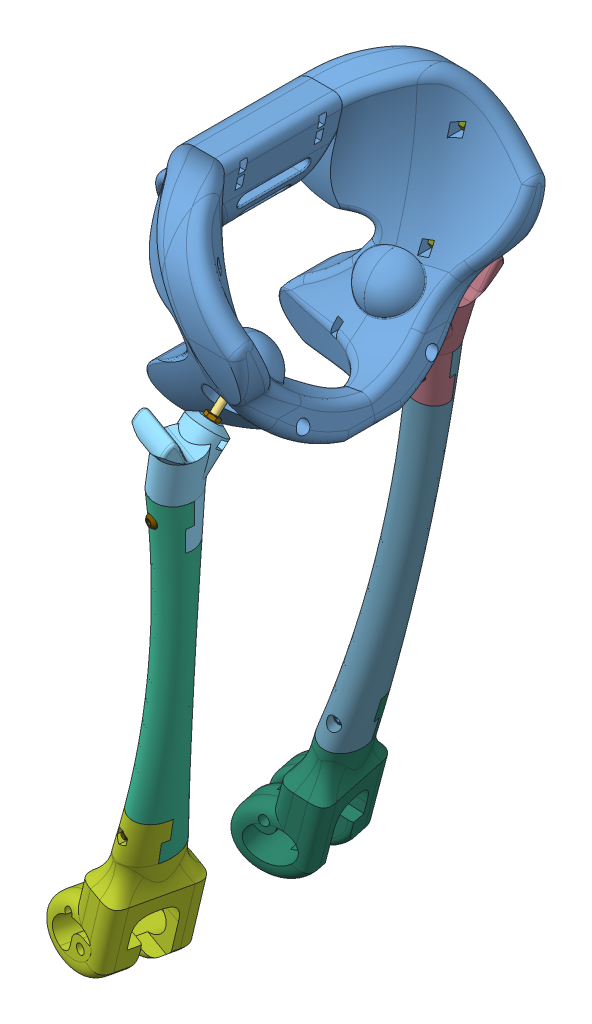
SolidWorks assembly Hips_VerticalCutVer10_Assembly, configuration Default. Lengths in mm.
Overall size (217.51 637.91 297.67).
53 component instances, 21 part files, 66 mates.
Components (placement in the parent):
- IliumRebuilt_Ver10-1: IliumRebuilt_Ver10 [Default] at origin size (197.88 220.17 282.18)
- Femoral_Head_ver1-1: Femoral_Head_ver1 [Default] at (17.9842 -18.1038 8.0845) x (0.971595 0.045629 0.232211) z (-0.227271 -0.093624 0.969321) size (39.5 39.5 39.5)
- 95327A531_HIGH-STRG ZINC YELLOW-CHROMATE PLTD CAP SCREW-1: 95327A531_HIGH-STRG ZINC YELLOW-CHROMATE PLTD CAP SCREW [95327A531] at (-63.8384 -68.3613 80.3964) x (-0.114057 -0.769464 0.628424) z (0.409289 0.539984 0.735459) size (49.38 11.55 10)
- Femoral_Head_Ver1_Cap-1: Femoral_Head_Ver1_Cap [Default] at (17.9868 -18.1069 8.0812) x (0.971595 0.045629 0.232211) z (-0.227271 -0.093624 0.969321) size (19.53 20.18 20.18)
- 03_02_Femoral_Head_Right-1: 03_02_Femoral_Head_Right [Default] at (-72.0104 -117.246 110.2958) x (-0.952156 0.241885 -0.186789) z (0.205625 0.054888 -0.97709) size (46.92 105.86 63.35)
- 03_03_Femur_Right-1: 03_03_Femur_Right [Default] at (-120.2542 -417.7721 83.261) x (-0.952156 0.241885 -0.186789) z (0.205625 0.054888 -0.97709) size (54.81 304.92 50.87)
- 05_01_Knee_Top-1: 05_01_Knee_Top [Default] at (-149.6638 -490.6352 77.3331) x (-0.952156 0.241885 -0.186789) z (0.185137 -0.029753 -0.982262) size (74.55 156.7 74.23)
- 94645A205_HIGH-STRENGTH STEEL NYLON-INSERT LOCKNUT-1: 94645A205_HIGH-STRENGTH STEEL NYLON-INSERT LOCKNUT [94645A205] at (-65.6633 -80.6727 90.4512) x (0.993354 -0.098188 0.060066) z (-0.015485 -0.631098 -0.775548) size (10 6.41 11.55)
- 90695A038_CLASS 04 STEEL THIN HEX NUT - DIN 439B-1: 90695A038_CLASS 04 STEEL THIN HEX NUT - DIN 439B [90695A038] at (-64.7965 -74.8248 85.6752) x (0.993328 -0.099162 0.058868) z (0.017019 0.630946 0.77564) size (10 3.98 11.55)
- MirrorFemoral_Head_ver1-2: MirrorFemoral_Head_ver1 [Default] at (17.9842 -18.1038 -8.0845) x (0.971595 0.045629 -0.232211) z (0.227271 0.093624 0.969321) size (39.5 39.5 39.5)
- Mirror95327A531_HIGH-STRG ZINC YELLOW-CHROMATE PLTD CAP SCREW-2: Mirror95327A531_HIGH-STRG ZINC YELLOW-CHROMATE PLTD CAP SCREW [95327A531] at (-63.8384 -68.3613 -80.3964) x (-0.114057 -0.769464 -0.628424) z (-0.409289 -0.539984 0.735459) size (49.38 11.55 10)
- MirrorFemoral_Head_Ver1_Cap-2: MirrorFemoral_Head_Ver1_Cap [Default] at (17.9868 -18.1069 -8.0812) x (0.971595 0.045629 -0.232211) z (0.227271 0.093624 0.969321) size (19.53 20.18 20.18)
- Mirror03_02_Femoral_Head_Right-2: Mirror03_02_Femoral_Head_Right [Default] at (-72.0104 -117.246 -110.2958) x (-0.952156 0.241885 0.186789) z (-0.205625 -0.054888 -0.97709) size (46.92 105.86 63.35)
- Mirror03_03_Femur_Right-2: Mirror03_03_Femur_Right [Default] at (-120.2542 -417.7721 -83.261) x (-0.952156 0.241885 0.186789) z (-0.205625 -0.054888 -0.97709) size (54.81 304.92 50.87)
- Mirror05_01_Knee_Top-2: Mirror05_01_Knee_Top [Default] at (-149.6638 -490.6352 -77.3331) x (-0.952156 0.241885 0.186789) z (-0.185137 0.029753 -0.982262) size (74.55 156.7 74.23)
- Mirror94645A205_HIGH-STRENGTH STEEL NYLON-INSERT LOCKNUT-2: Mirror94645A205_HIGH-STRENGTH STEEL NYLON-INSERT LOCKNUT [94645A205] at (-65.6633 -80.6727 -90.4512) x (0.993354 -0.098188 -0.060066) z (0.015485 0.631098 -0.775548) size (10 6.41 11.55)
- Mirror90695A038_CLASS 04 STEEL THIN HEX NUT - DIN 439B-2: Mirror90695A038_CLASS 04 STEEL THIN HEX NUT - DIN 439B [90695A038] at (-64.7965 -74.8248 -85.6752) x (0.993328 -0.099162 -0.058868) z (-0.017019 -0.630946 0.77564) size (10 3.98 11.55)
- 91239A330_CLASS 10.9 STL BUTTON-HEAD SOCKET CAP SCREW-1: 91239A330_CLASS 10.9 STL BUTTON-HEAD SOCKET CAP SCREW [91239A330] at (-44.244 -75.4386 54.7323) x (0 0 -1) z (1 0 0) size (10.5 10.5 38.95)
- 91239A330_CLASS 10.9 STL BUTTON-HEAD SOCKET CAP SCREW-4: 91239A330_CLASS 10.9 STL BUTTON-HEAD SOCKET CAP SCREW [91239A330] at (-77.844 52.8275 110.8479) x (0 -0.939693 0.34202) z (-1 0 0) size (10.5 10.5 38.95)
- 91239A330_CLASS 10.9 STL BUTTON-HEAD SOCKET CAP SCREW-6: 91239A330_CLASS 10.9 STL BUTTON-HEAD SOCKET CAP SCREW [91239A330] at (-77.844 -21.0136 84.8541) x (0 -0.866025 0.5) z (-1 0 0) size (10.5 10.5 38.95)
- 91239A330_CLASS 10.9 STL BUTTON-HEAD SOCKET CAP SCREW-8: 91239A330_CLASS 10.9 STL BUTTON-HEAD SOCKET CAP SCREW [91239A330] at (-121.884 56.6312 66.8) x (0.173648 0.984808 0) z (0 0 1) size (10.5 10.5 38.95)
- 91239A330_CLASS 10.9 STL BUTTON-HEAD SOCKET CAP SCREW-10: 91239A330_CLASS 10.9 STL BUTTON-HEAD SOCKET CAP SCREW [91239A330] at (-104.3146 69.6752 66.8) x (-0.173648 0.984808 0) z (0 0 1) size (10.5 10.5 38.95)
- 91239A330_CLASS 10.9 STL BUTTON-HEAD SOCKET CAP SCREW-13: 91239A330_CLASS 10.9 STL BUTTON-HEAD SOCKET CAP SCREW [91239A330] at (-76.9699 -137.6299 128.1216) x (-0.583019 0.808777 -0.077261) z (-0.205625 -0.054888 0.97709) size (10.5 10.5 38.95)
- 91239A330_CLASS 10.9 STL BUTTON-HEAD SOCKET CAP SCREW-15: 91239A330_CLASS 10.9 STL BUTTON-HEAD SOCKET CAP SCREW [91239A330] at (-112.4792 -398.3917 68.7251) x (-0.97858 0.021691 -0.20472) z (0.205625 0.054888 -0.97709) size (10.5 10.5 38.95)
- Mirror91239A330_CLASS 10.9 STL BUTTON-HEAD SOCKET CAP SCREW-17: Mirror91239A330_CLASS 10.9 STL BUTTON-HEAD SOCKET CAP SCREW [91239A330] at (-44.244 -75.4386 -54.7323) x (0 0 1) z (-1 0 0) size (10.5 10.5 38.95)
- Mirror91239A330_CLASS 10.9 STL BUTTON-HEAD SOCKET CAP SCREW-18: Mirror91239A330_CLASS 10.9 STL BUTTON-HEAD SOCKET CAP SCREW [91239A330] at (-77.844 52.8275 -110.8479) x (0 -0.939693 -0.34202) z (1 0 0) size (10.5 10.5 38.95)
- Mirror91239A330_CLASS 10.9 STL BUTTON-HEAD SOCKET CAP SCREW-19: Mirror91239A330_CLASS 10.9 STL BUTTON-HEAD SOCKET CAP SCREW [91239A330] at (-121.884 56.6312 -66.8) x (0.173648 0.984808 0) z (0 0 1) size (10.5 10.5 38.95)
- Mirror91239A330_CLASS 10.9 STL BUTTON-HEAD SOCKET CAP SCREW-20: Mirror91239A330_CLASS 10.9 STL BUTTON-HEAD SOCKET CAP SCREW [91239A330] at (-77.844 -21.0136 -84.8541) x (0 -0.866025 -0.5) z (1 0 0) size (10.5 10.5 38.95)
- Mirror91239A330_CLASS 10.9 STL BUTTON-HEAD SOCKET CAP SCREW-21: Mirror91239A330_CLASS 10.9 STL BUTTON-HEAD SOCKET CAP SCREW [91239A330] at (-104.3146 69.6752 -66.8) x (-0.173648 0.984808 0) z (0 0 1) size (10.5 10.5 38.95)
- Mirror91239A330_CLASS 10.9 STL BUTTON-HEAD SOCKET CAP SCREW-22: Mirror91239A330_CLASS 10.9 STL BUTTON-HEAD SOCKET CAP SCREW [91239A330] at (-112.4792 -398.3917 -68.7251) x (-0.97858 0.021691 0.20472) z (-0.205625 -0.054888 -0.97709) size (10.5 10.5 38.95)
- Mirror91239A330_CLASS 10.9 STL BUTTON-HEAD SOCKET CAP SCREW-23: Mirror91239A330_CLASS 10.9 STL BUTTON-HEAD SOCKET CAP SCREW [91239A330] at (-76.9699 -137.6299 -128.1216) x (-0.583019 0.808777 0.077261) z (0.205625 0.054888 0.97709) size (10.5 10.5 38.95)
- 94645A205_HIGH-STRENGTH STEEL NYLON-INSERT LOCKNUT-2: 94645A205_HIGH-STRENGTH STEEL NYLON-INSERT LOCKNUT [94645A205] at (-47.544 52.8275 110.8479) x (0 -1 0) z (0 0 1) size (10 6.41 11.55)
- 94645A205_HIGH-STRENGTH STEEL NYLON-INSERT LOCKNUT-3: 94645A205_HIGH-STRENGTH STEEL NYLON-INSERT LOCKNUT [94645A205] at (-47.544 -21.0136 84.8541) x (0 -1 0) z (0 0 1) size (10 6.41 11.55)
- 94645A205_HIGH-STRENGTH STEEL NYLON-INSERT LOCKNUT-5: 94645A205_HIGH-STRENGTH STEEL NYLON-INSERT LOCKNUT [94645A205] at (-81.044 -75.4386 54.7323) x (0 1 0) z (0 0 -1) size (10 6.41 11.55)
- 94645A205_HIGH-STRENGTH STEEL NYLON-INSERT LOCKNUT-7: 94645A205_HIGH-STRENGTH STEEL NYLON-INSERT LOCKNUT [94645A205] at (-104.3146 69.6752 36.5) x (0 -1 0) z (1 0 0) size (10 6.41 11.55)
- 94645A205_HIGH-STRENGTH STEEL NYLON-INSERT LOCKNUT-9: 94645A205_HIGH-STRENGTH STEEL NYLON-INSERT LOCKNUT [94645A205] at (-121.884 56.6312 36.5) x (0 -1 0) z (1 0 0) size (10 6.41 11.55)
- 94645A205_HIGH-STRENGTH STEEL NYLON-INSERT LOCKNUT-13: 94645A205_HIGH-STRENGTH STEEL NYLON-INSERT LOCKNUT [94645A205] at (-70.5984 -135.9292 97.8454) x (0.711546 -0.693854 0.110765) z (0.671879 0.71802 0.181729) size (10 6.41 11.55)
- 94645A205_HIGH-STRENGTH STEEL NYLON-INSERT LOCKNUT-15: 94645A205_HIGH-STRENGTH STEEL NYLON-INSERT LOCKNUT [94645A205] at (-118.6418 -400.0367 98.0085) x (-0.952156 0.241885 -0.186789) z (0.226091 0.968751 0.102) size (10 6.41 11.55)
- 94645A205_HIGH-STRENGTH STEEL NYLON-INSERT LOCKNUT-11: 94645A205_HIGH-STRENGTH STEEL NYLON-INSERT LOCKNUT [94645A205] at (-30.2115 -92.3012 -13.5) x (0 -1 0) z (1 0 0) size (10 6.41 11.55)
- 91239A330_CLASS 10.9 STL BUTTON-HEAD SOCKET CAP SCREW-24: 91239A330_CLASS 10.9 STL BUTTON-HEAD SOCKET CAP SCREW [91239A330] at (-30.2115 -92.3012 16.8) x (0.925851 0.377888 0) z (0 0 1) size (10.5 10.5 38.95)
- Mirror94645A205_HIGH-STRENGTH STEEL NYLON-INSERT LOCKNUT-13: Mirror94645A205_HIGH-STRENGTH STEEL NYLON-INSERT LOCKNUT [94645A205] at (-47.544 52.8275 -110.8479) x (0 -1 0) z (0 0 1) size (10 6.41 11.55)
- Mirror94645A205_HIGH-STRENGTH STEEL NYLON-INSERT LOCKNUT-14: Mirror94645A205_HIGH-STRENGTH STEEL NYLON-INSERT LOCKNUT [94645A205] at (-47.544 -21.0136 -84.8541) x (0 -1 0) z (0 0 1) size (10 6.41 11.55)
- Mirror94645A205_HIGH-STRENGTH STEEL NYLON-INSERT LOCKNUT-15: Mirror94645A205_HIGH-STRENGTH STEEL NYLON-INSERT LOCKNUT [94645A205] at (-81.044 -75.4386 -54.7323) x (0 1 0) z (0 0 -1) size (10 6.41 11.55)
- Mirror94645A205_HIGH-STRENGTH STEEL NYLON-INSERT LOCKNUT-16: Mirror94645A205_HIGH-STRENGTH STEEL NYLON-INSERT LOCKNUT [94645A205] at (-104.3146 69.6752 -36.5) x (0 -1 0) z (-1 0 0) size (10 6.41 11.55)
- Mirror94645A205_HIGH-STRENGTH STEEL NYLON-INSERT LOCKNUT-17: Mirror94645A205_HIGH-STRENGTH STEEL NYLON-INSERT LOCKNUT [94645A205] at (-121.884 56.6312 -36.5) x (0 -1 0) z (-1 0 0) size (10 6.41 11.55)
- Mirror94645A205_HIGH-STRENGTH STEEL NYLON-INSERT LOCKNUT-18: Mirror94645A205_HIGH-STRENGTH STEEL NYLON-INSERT LOCKNUT [94645A205] at (-70.5984 -135.9292 -97.8454) x (0.711546 -0.693854 -0.110765) z (-0.671879 -0.71802 0.181729) size (10 6.41 11.55)
- Mirror94645A205_HIGH-STRENGTH STEEL NYLON-INSERT LOCKNUT-19: Mirror94645A205_HIGH-STRENGTH STEEL NYLON-INSERT LOCKNUT [94645A205] at (-118.6418 -400.0367 -98.0085) x (-0.952156 0.241885 0.186789) z (-0.226091 -0.968751 0.102) size (10 6.41 11.55)
- 91595A476_METRIC ALLOY STEEL DOWEL PIN-1: 91595A476_METRIC ALLOY STEEL DOWEL PIN [91595A476] at (-61.544 24.9417 100.1676) x (1 0 0) z (0 0.977288 -0.211915) size (40 6 6)
- 91595A476_METRIC ALLOY STEEL DOWEL PIN-2: 91595A476_METRIC ALLOY STEEL DOWEL PIN [91595A476] at (-61.544 -3.0834 90.0569) x (1 0 0) z (0 0.998526 -0.054283) size (40 6 6)
- 91595A476_METRIC ALLOY STEEL DOWEL PIN-4: 91595A476_METRIC ALLOY STEEL DOWEL PIN [91595A476] at (-61.544 -93.1682 40.0283) x (1 0 0) z (0 0.99731 0.073303) size (40 6 6)
- Mirror91595A476_METRIC ALLOY STEEL DOWEL PIN-6: Mirror91595A476_METRIC ALLOY STEEL DOWEL PIN [91595A476] at (-61.544 24.9417 -100.1676) x (1 0 0) z (0 -0.977288 -0.211915) size (40 6 6)
- Mirror91595A476_METRIC ALLOY STEEL DOWEL PIN-7: Mirror91595A476_METRIC ALLOY STEEL DOWEL PIN [91595A476] at (-61.544 -3.0834 -90.0569) x (1 0 0) z (0 -0.998526 -0.054283) size (40 6 6)
- Mirror91595A476_METRIC ALLOY STEEL DOWEL PIN-8: Mirror91595A476_METRIC ALLOY STEEL DOWEL PIN [91595A476] at (-61.544 -93.1682 -40.0283) x (1 0 0) z (0 -0.99731 0.073303) size (40 6 6)
Mates (geometry in assembly coordinates):
- Coincident1: coincident anti-aligned: plane of Femoral_Head_ver1-1 through (10.1204 -71.1554 51.412) normal (-0.114057 -0.769464 0.628424); plane of 95327A531_HIGH-STRG ZINC YELLOW-CHROMATE PLTD CAP SCREW-1 through (-65.7037 -51.2247 62.054) normal (0.114057 0.769464 -0.628424)
- Concentric1: concentric anti-aligned: cylinder of Femoral_Head_ver1-1 through (-64.2297 -71.0011 82.5523) axis (0.114057 0.769464 -0.628424) radius 3.25; cylinder of 95327A531_HIGH-STRG ZINC YELLOW-CHROMATE PLTD CAP SCREW-1 through (-61.5002 -52.5873 67.5137) axis (-0.114057 -0.769464 0.628424) radius 3
- Coincident2: coincident anti-aligned: plane of Femoral_Head_ver1-1 through (10.1204 -71.1554 51.412) normal (-0.114057 -0.769464 0.628424); plane of Femoral_Head_Ver1_Cap-1 through (-43.1095 -44.7494 74.0834) normal (0.114057 0.769464 -0.628424)
- Coincident3: coincident: line of Femoral_Head_ver1-1 through (-44.9277 -48.1631 76.3365) axis (-0.971595 -0.045629 -0.232211); plane of Femoral_Head_Ver1_Cap-1 through (-62.2868 -45.8264 69.483) normal (-0.207353 0.637059 0.742402)
- Coincident4: coincident: circle of Femoral_Head_ver1-1; point of Femoral_Head_Ver1_Cap-1
- Concentric5: concentric: sphere of IliumRebuilt_Ver10-1; sphere of Femoral_Head_ver1-1
- Concentric8: concentric anti-aligned: cylinder of 95327A531_HIGH-STRG ZINC YELLOW-CHROMATE PLTD CAP SCREW-1 through (-61.5002 -52.5873 67.5137) axis (-0.114057 -0.769464 0.628424) radius 3; cylinder of 03_02_Femoral_Head_Right-1 through (-66.6328 -87.2132 95.7928) axis (0.114057 0.769464 -0.628424) radius 3.125
- Coincident5: coincident anti-aligned: plane of 95327A531_HIGH-STRG ZINC YELLOW-CHROMATE PLTD CAP SCREW-1 through (-66.6328 -87.2132 95.7928) normal (-0.114057 -0.769464 0.628424); circle of 03_02_Femoral_Head_Right-1
- Coincident6: coincident anti-aligned: plane of 03_02_Femoral_Head_Right-1 through (-72.0104 -117.246 110.2958) normal (-0.226091 -0.968751 -0.102); plane of 03_03_Femur_Right-1 through (-72.0103 -117.2461 110.2958) normal (0.226091 0.968751 0.102)
- Coincident7: coincident anti-aligned: plane of 03_02_Femoral_Head_Right-1 through (-34.2234 -126.4394 113.8522) normal (-0.205625 -0.054888 0.97709); plane of 03_03_Femur_Right-1 through (-103.1296 -421.7164 82.7639) normal (0.205625 0.054888 -0.97709)
- Coincident8: coincident: point of 03_02_Femoral_Head_Right-1; point of 03_03_Femur_Right-1
- Coincident9: coincident anti-aligned: plane of 03_03_Femur_Right-1 through (-95.2949 -385.015 90.3537) normal (-0.226091 -0.968751 -0.102); plane of 05_01_Knee_Top-1 through (-92.2857 -386.2352 95.2728) normal (0.226091 0.968751 0.102)
- Coincident10: coincident anti-aligned: plane of 03_03_Femur_Right-1 through (-103.4699 -421.8072 84.381) normal (-0.205625 -0.054888 0.97709); plane of 05_01_Knee_Top-1 through (-117.1848 -498.2016 77.2033) normal (0.205625 0.054888 -0.97709)
- Coincident11: coincident: point of 03_03_Femur_Right-1; point of 05_01_Knee_Top-1
- Coincident12: coincident anti-aligned: plane of 03_02_Femoral_Head_Right-1 through (-67.2957 -85.439 84.3189) normal (-0.114057 -0.769464 0.628424); plane of 94645A205_HIGH-STRENGTH STEEL NYLON-INSERT LOCKNUT-1 through (-60.6518 -79.3418 92.9903) normal (0.114057 0.769464 -0.628424)
- Concentric9: concentric anti-aligned: cylinder of 95327A531_HIGH-STRG ZINC YELLOW-CHROMATE PLTD CAP SCREW-1 through (-61.5002 -52.5873 67.5137) axis (-0.114057 -0.769464 0.628424) radius 3; circle of 94645A205_HIGH-STRENGTH STEEL NYLON-INSERT LOCKNUT-1
- Coincident13: coincident anti-aligned: plane of 03_02_Femoral_Head_Right-1 through (-64.9789 -76.0559 86.6806) normal (0.114057 0.769464 -0.628424); plane of 90695A038_CLASS 04 STEEL THIN HEX NUT - DIN 439B-1 through (-69.9947 -77.3815 84.1472) normal (-0.114057 -0.769464 0.628424)
- Coincident14: coincident anti-aligned: cylinder of 95327A531_HIGH-STRG ZINC YELLOW-CHROMATE PLTD CAP SCREW-1 through (-61.5002 -52.5873 67.5137) axis (-0.114057 -0.769464 0.628424) radius 3; circle of 90695A038_CLASS 04 STEEL THIN HEX NUT - DIN 439B-1
- Concentric10: concentric aligned: cylinder of IliumRebuilt_Ver10-1 through (18.4173 -75.4386 54.7323) axis (-1 0 0) radius 5.375; cylinder of 91239A330_CLASS 10.9 STL BUTTON-HEAD SOCKET CAP SCREW-1 through (-82.544 -75.4386 54.7323) axis (-1 0 0) radius 3
- Coincident15: coincident anti-aligned: plane of IliumRebuilt_Ver10-1 through (-47.544 -75.4386 54.7323) normal (1 0 0); plane of 91239A330_CLASS 10.9 STL BUTTON-HEAD SOCKET CAP SCREW-1 through (-47.544 -80.6886 54.7323) normal (-1 0 0)
- Concentric11: concentric aligned: cylinder of IliumRebuilt_Ver10-1 through (18.4173 -75.4386 -54.7323) axis (-1 0 0) radius 5.375; cylinder of 91239A330_CLASS 10.9 STL BUTTON-HEAD SOCKET CAP SCREW-2 through (-82.544 -75.4011 -54.6673) axis (-1 0 0) radius 3
- Coincident16: coincident anti-aligned: plane of IliumRebuilt_Ver10-1 through (-47.544 -75.4386 -54.7323) normal (1 0 0); plane of 91239A330_CLASS 10.9 STL BUTTON-HEAD SOCKET CAP SCREW-2 through (-47.544 -80.5847 -55.4997) normal (-1 0 0)
- Concentric12: concentric aligned: cylinder of IliumRebuilt_Ver10-1 through (-187.4808 52.8275 110.8479) axis (1 0 0) radius 5.375; cylinder of 91239A330_CLASS 10.9 STL BUTTON-HEAD SOCKET CAP SCREW-4 through (-39.544 52.8275 110.8479) axis (1 0 0) radius 3
- Coincident17: coincident anti-aligned: plane of IliumRebuilt_Ver10-1 through (-74.544 52.8275 110.8479) normal (-1 0 0); plane of 91239A330_CLASS 10.9 STL BUTTON-HEAD SOCKET CAP SCREW-4 through (-74.544 51.0319 105.9145) normal (1 0 0)
- Concentric13: concentric aligned: cylinder of IliumRebuilt_Ver10-1 through (-187.4808 -21.0136 84.8541) axis (1 0 0) radius 5.375; cylinder of 91239A330_CLASS 10.9 STL BUTTON-HEAD SOCKET CAP SCREW-6 through (-39.544 -21.0136 84.8541) axis (1 0 0) radius 3
- Coincident18: coincident anti-aligned: plane of IliumRebuilt_Ver10-1 through (-74.544 -21.0136 84.8541) normal (-1 0 0); plane of 91239A330_CLASS 10.9 STL BUTTON-HEAD SOCKET CAP SCREW-6 through (-74.544 -23.6386 80.3075) normal (1 0 0)
- Concentric14: concentric aligned: cylinder of IliumRebuilt_Ver10-1 through (-121.884 56.6312 143.5354) axis (0 0 -1) radius 5.375; cylinder of 91239A330_CLASS 10.9 STL BUTTON-HEAD SOCKET CAP SCREW-8 through (-121.884 56.6312 28.5) axis (0 0 -1) radius 3
- Coincident19: coincident anti-aligned: plane of IliumRebuilt_Ver10-1 through (-121.884 56.6312 63.5) normal (0 0 1); plane of 91239A330_CLASS 10.9 STL BUTTON-HEAD SOCKET CAP SCREW-8 through (-116.7138 55.7195 63.5) normal (0 0 -1)
- Concentric15: concentric aligned: cylinder of IliumRebuilt_Ver10-1 through (-104.3146 69.6752 143.5354) axis (0 0 -1) radius 5.375; cylinder of 91239A330_CLASS 10.9 STL BUTTON-HEAD SOCKET CAP SCREW-10 through (-104.3146 69.6752 28.5) axis (0 0 -1) radius 3
- Coincident20: coincident anti-aligned: plane of IliumRebuilt_Ver10-1 through (-104.3146 69.6752 63.5) normal (0 0 1); plane of 91239A330_CLASS 10.9 STL BUTTON-HEAD SOCKET CAP SCREW-10 through (-99.1443 70.5868 63.5) normal (0 0 -1)
- Concentric16: concentric aligned: cylinder of 03_03_Femur_Right-1 through (-78.1748 -137.9516 133.8471) axis (0.205625 0.054888 -0.97709) radius 5.5; cylinder of 91239A330_CLASS 10.9 STL BUTTON-HEAD SOCKET CAP SCREW-13 through (-69.0945 -135.5277 90.699) axis (0.205625 0.054888 -0.97709) radius 3
- Coincident21: coincident anti-aligned: plane of 03_03_Femur_Right-1 through (-76.2914 -137.4488 124.8972) normal (-0.205625 -0.054888 0.97709); plane of 91239A330_CLASS 10.9 STL BUTTON-HEAD SOCKET CAP SCREW-13 through (-72.1648 -134.3747 125.9383) normal (0.205625 0.054888 -0.97709)
- Concentric17: concentric aligned: cylinder of 03_03_Femur_Right-1 through (-110.7122 -397.92 60.3286) axis (-0.205625 -0.054888 0.97709) radius 5.5; cylinder of 91239A330_CLASS 10.9 STL BUTTON-HEAD SOCKET CAP SCREW-15 through (-120.3547 -400.4939 106.1476) axis (-0.205625 -0.054888 0.97709) radius 3
- Coincident22: coincident anti-aligned: plane of 03_03_Femur_Right-1 through (-113.1578 -398.5728 71.9495) normal (0.205625 0.054888 -0.97709); plane of 91239A330_CLASS 10.9 STL BUTTON-HEAD SOCKET CAP SCREW-15 through (-113.2101 -403.8136 71.6441) normal (-0.205625 -0.054888 0.97709)
- Concentric18: concentric anti-aligned: circle of IliumRebuilt_Ver10-1; circle of 94645A205_HIGH-STRENGTH STEEL NYLON-INSERT LOCKNUT-2
- Coincident23: coincident anti-aligned: plane of IliumRebuilt_Ver10-1 through (-47.544 0 0) normal (1 0 0); plane of 94645A205_HIGH-STRENGTH STEEL NYLON-INSERT LOCKNUT-2 through (-47.544 47.8275 107.9612) normal (-1 0 0)
- Parallel1: parallel anti-aligned: plane of IliumRebuilt_Ver10-1 through (-41.044 57.9775 107.8746) normal (0 -1 0); plane of 94645A205_HIGH-STRENGTH STEEL NYLON-INSERT LOCKNUT-2 through (-41.544 57.8275 107.9612) normal (0 1 0)
- Concentric19: concentric anti-aligned: circle of IliumRebuilt_Ver10-1; circle of 94645A205_HIGH-STRENGTH STEEL NYLON-INSERT LOCKNUT-3
- Coincident25: coincident anti-aligned: plane of IliumRebuilt_Ver10-1 through (-47.544 0 0) normal (1 0 0); plane of 94645A205_HIGH-STRENGTH STEEL NYLON-INSERT LOCKNUT-3 through (-47.544 -26.0136 81.9674) normal (-1 0 0)
- Parallel2: parallel anti-aligned: plane of IliumRebuilt_Ver10-1 through (-41.044 -15.8636 81.8808) normal (0 -1 0); plane of 94645A205_HIGH-STRENGTH STEEL NYLON-INSERT LOCKNUT-3 through (-41.544 -16.0136 81.9674) normal (0 1 0)
- Concentric20: concentric anti-aligned: circle of IliumRebuilt_Ver10-1; circle of 94645A205_HIGH-STRENGTH STEEL NYLON-INSERT LOCKNUT-5
- Coincident26: coincident anti-aligned: plane of IliumRebuilt_Ver10-1 through (-81.044 0 0) normal (1 0 0); plane of 94645A205_HIGH-STRENGTH STEEL NYLON-INSERT LOCKNUT-5 through (-81.044 -70.4386 57.619) normal (-1 0 0)
- Parallel3: parallel anti-aligned: plane of IliumRebuilt_Ver10-1 through (-81.044 -80.5886 57.7056) normal (0 1 0); plane of 94645A205_HIGH-STRENGTH STEEL NYLON-INSERT LOCKNUT-5 through (-75.044 -80.4386 57.619) normal (0 -1 0)
- Concentric21: concentric anti-aligned: circle of IliumRebuilt_Ver10-1; circle of 94645A205_HIGH-STRENGTH STEEL NYLON-INSERT LOCKNUT-7
- Coincident27: coincident anti-aligned: plane of IliumRebuilt_Ver10-1 through (0 0 36.5) normal (0 0 -1); plane of 94645A205_HIGH-STRENGTH STEEL NYLON-INSERT LOCKNUT-7 through (-107.2013 64.6752 36.5) normal (0 0 1)
- Parallel4: parallel anti-aligned: plane of IliumRebuilt_Ver10-1 through (-107.2879 74.8252 30.5) normal (0 -1 0); plane of 94645A205_HIGH-STRENGTH STEEL NYLON-INSERT LOCKNUT-7 through (-107.2013 74.6752 30.5) normal (0 1 0)
- Concentric22: concentric anti-aligned: circle of IliumRebuilt_Ver10-1; circle of 94645A205_HIGH-STRENGTH STEEL NYLON-INSERT LOCKNUT-9
- Coincident28: coincident anti-aligned: plane of IliumRebuilt_Ver10-1 through (0 0 36.5) normal (0 0 -1); plane of 94645A205_HIGH-STRENGTH STEEL NYLON-INSERT LOCKNUT-9 through (-124.7708 51.6312 36.5) normal (0 0 1)
- Parallel5: parallel anti-aligned: plane of IliumRebuilt_Ver10-1 through (-124.8574 61.7812 30.5) normal (0 -1 0); plane of 94645A205_HIGH-STRENGTH STEEL NYLON-INSERT LOCKNUT-9 through (-124.7708 61.6312 30.5) normal (0 1 0)
- Concentric23: concentric aligned: circle of IliumRebuilt_Ver10-1; circle of 94645A205_HIGH-STRENGTH STEEL NYLON-INSERT LOCKNUT-11
- Coincident29: coincident anti-aligned: plane of IliumRebuilt_Ver10-1 through (0 0 -13.5) normal (0 0 -1); plane of 94645A205_HIGH-STRENGTH STEEL NYLON-INSERT LOCKNUT-11 through (-33.0982 -97.3012 -13.5) normal (0 0 1)
- Parallel6: parallel anti-aligned: plane of IliumRebuilt_Ver10-1 through (-33.1848 -87.1512 -143.5354) normal (0 -1 0); plane of 94645A205_HIGH-STRENGTH STEEL NYLON-INSERT LOCKNUT-11 through (-33.0982 -87.3012 -19.5) normal (0 1 0)
- Concentric24: concentric aligned: cylinder of IliumRebuilt_Ver10-1 through (-30.2115 -92.3012 143.5354) axis (0 0 -1) radius 5.375; cylinder of 91239A330_CLASS 10.9 STL BUTTON-HEAD SOCKET CAP SCREW-24 through (-30.2115 -92.3012 -21.5) axis (0 0 -1) radius 3
- Coincident30: coincident anti-aligned: plane of IliumRebuilt_Ver10-1 through (0 0 13.5) normal (0 0 1); plane of 91239A330_CLASS 10.9 STL BUTTON-HEAD SOCKET CAP SCREW-24 through (-28.2276 -97.1619 13.5) normal (0 0 -1)
- Concentric25: concentric aligned: circle of 03_02_Femoral_Head_Right-1; circle of 94645A205_HIGH-STRENGTH STEEL NYLON-INSERT LOCKNUT-13
- Coincident31: coincident anti-aligned: plane of 03_02_Femoral_Head_Right-1 through (-69.6601 -116.6187 99.1276) normal (0.205625 0.054888 -0.97709); plane of 94645A205_HIGH-STRENGTH STEEL NYLON-INSERT LOCKNUT-13 through (-68.9802 -141.4712 97.8746) normal (-0.205625 -0.054888 0.97709)
- Parallel7: parallel anti-aligned: plane of 03_02_Femoral_Head_Right-1 through (-74.7916 -134.0414 89.2104) normal (0.711546 -0.693854 0.110765); plane of 94645A205_HIGH-STRENGTH STEEL NYLON-INSERT LOCKNUT-13 through (-74.8619 -134.2033 90.9044) normal (-0.711546 0.693854 -0.110765)
- Concentric26: concentric aligned: circle of 05_01_Knee_Top-1; circle of 94645A205_HIGH-STRENGTH STEEL NYLON-INSERT LOCKNUT-15
- Coincident32: coincident anti-aligned: plane of 05_01_Knee_Top-1 through (-151.4835 -491.121 85.9804) normal (-0.205625 -0.054888 0.97709); plane of 94645A205_HIGH-STRENGTH STEEL NYLON-INSERT LOCKNUT-15 through (-124.0552 -401.6238 96.7801) normal (0.205625 0.054888 -0.97709)
- Parallel8: parallel anti-aligned: plane of 05_01_Knee_Top-1 through (-119.4386 -400.1002 130.0943) normal (-0.952156 0.241885 -0.186789); plane of 94645A205_HIGH-STRENGTH STEEL NYLON-INSERT LOCKNUT-15 through (-115.7674 -404.372 104.5105) normal (0.952156 -0.241885 0.186789)
- Concentric27: concentric anti-aligned: circle of IliumRebuilt_Ver10-1; circle of 91595A476_METRIC ALLOY STEEL DOWEL PIN-1
- Coincident33: coincident: plane of IliumRebuilt_Ver10-1 through (-81.544 24.9417 100.1676) normal (1 0 0); point of 91595A476_METRIC ALLOY STEEL DOWEL PIN-1
- Concentric29: concentric anti-aligned: circle of IliumRebuilt_Ver10-1; circle of 91595A476_METRIC ALLOY STEEL DOWEL PIN-2
- Coincident34: coincident: plane of IliumRebuilt_Ver10-1 through (-81.544 -3.0834 90.0569) normal (1 0 0); point of 91595A476_METRIC ALLOY STEEL DOWEL PIN-2
- Concentric30: concentric anti-aligned: circle of IliumRebuilt_Ver10-1; circle of 91595A476_METRIC ALLOY STEEL DOWEL PIN-4
- Coincident35: coincident: plane of IliumRebuilt_Ver10-1 through (-81.544 -93.1682 40.0283) normal (1 0 0); point of 91595A476_METRIC ALLOY STEEL DOWEL PIN-4
